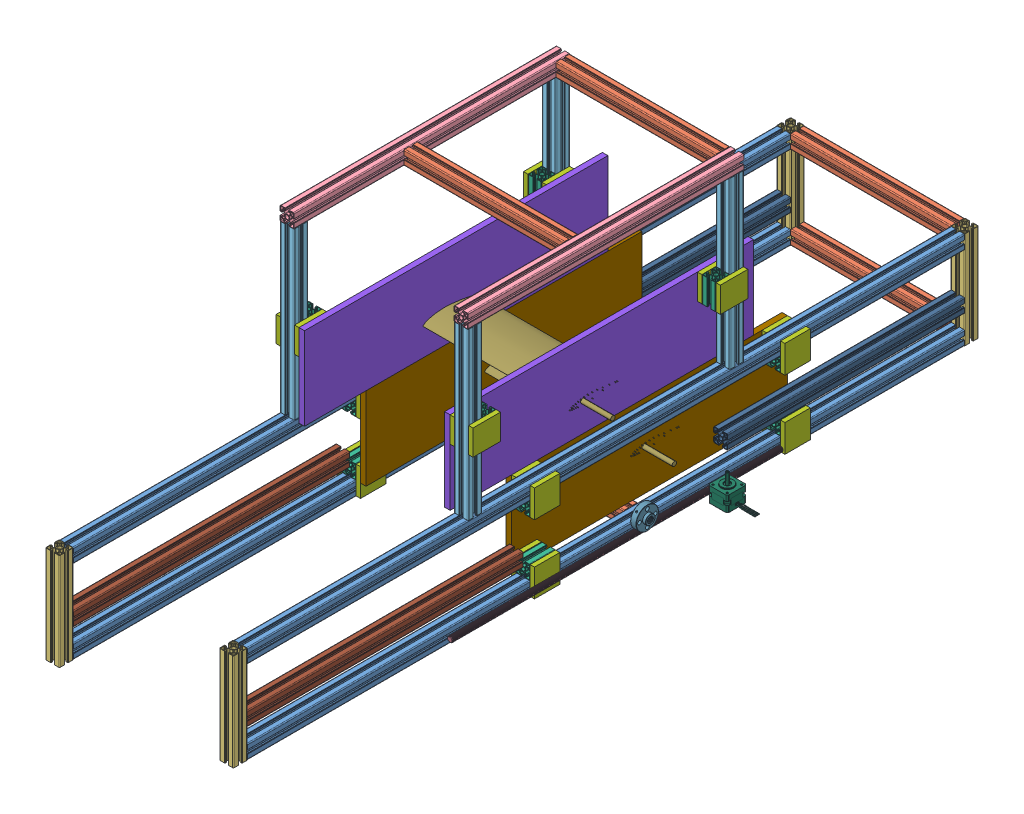
SolidWorks assembly Full Frame - Jack, configuration Default. Lengths in mm.
Overall size (567.71 501.2 1350.8).
82 component instances, 15 part files, 75 mates.
Components (placement in the parent):
- Stagger Frame-1: Stagger Frame [Default] at (96.6747 -83.0569 126.4787) size (340.8 175.8 1350.8)
  - Stagger - 1300x-1: Stagger - 1300x [Default] at (686.0911 649.1244 261.7798) size (25.4 25.4 1300)
  - Stagger - 1300x-2: Stagger - 1300x [Default] at (370.692 799.5238 261.7798) size (25.4 25.4 1300)
  - Stagger - 1300x-3: Stagger - 1300x [Default] at (686.0911 799.5238 261.7798) size (25.4 25.4 1300)
  - Stagger - 1300x-4: Stagger - 1300x [Default] at (370.692 649.1244 261.7798) size (25.4 25.4 1300)
  - Gap-220z-2: Gap-220z [Default] at (785.2806 799.5238 750.6531) x (0 0 1) z (-1 0 0) size (25.4 25.4 290)
  - Gap-220z-4: Gap-220z [Default] at (785.2806 649.1244 750.6531) x (0 0 1) z (-1 0 0) size (25.4 25.4 290)
  - Stagger 125y-5: Stagger 125y [Default] at (686.0911 880.052 750.6531) x (1 0 0) z (0 -1 0) size (25.4 25.4 175.8)
  - Stagger 125y-6: Stagger 125y [Default] at (370.692 880.052 750.6531) x (1 0 0) z (0 -1 0) size (25.4 25.4 175.8)
  - Stagger 125y-7: Stagger 125y [Default] at (370.692 568.5962 2076.0491) x (1 0 0) z (0 1 0) size (25.4 25.4 175.8)
  - Stagger 125y-8: Stagger 125y [Default] at (686.0911 568.5962 2076.0491) x (1 0 0) z (0 1 0) size (25.4 25.4 175.8)
- Gap Frame-1: Gap Frame [Default] at (534.4751 780.2503 996.128) size (340.8 325.4 500)
  - Gap-500x-1: Gap-500x [Default] at (248.2908 261.6156 100.7911) size (25.4 25.4 500)
  - Gap-500x-2: Gap-500x [Default] at (-67.1083 261.6156 100.7911) size (25.4 25.4 500)
  - Gap-300y-1: Gap-300y [Default] at (-67.1083 -166.8311 781.0023) x (1 0 0) z (0 1 0) size (25.4 25.4 300)
  - Gap-300y-2: Gap-300y [Default] at (-67.1083 -166.8311 306.4039) x (1 0 0) z (0 1 0) size (25.4 25.4 300)
  - Gap-300y-3: Gap-300y [Default] at (248.2908 364.6633 781.0023) x (1 0 0) z (0 -1 0) size (25.4 25.4 300)
  - Gap-300y-4: Gap-300y [Default] at (248.2908 364.6633 306.4039) x (1 0 0) z (0 -1 0) size (25.4 25.4 300)
  - Gap-220z-1: Gap-220z [Default] at (-166.2977 261.6156 581.8039) x (0 0 -1) z (1 0 0) size (25.4 25.4 290)
  - Gap-220z-2: Gap-220z [Default] at (347.4802 261.6156 306.4039) x (0 0 1) z (-1 0 0) size (25.4 25.4 290)
- Slider-1: Slider [Default] at (768.5368 912.233 1726.2246) x (1 0 0) z (0 -1 0) size (41.4 50 46)
  - Slider base-1: Slider base [Default] at (14.2291 25.5057 16.1181) size (25.4 25.4 46)
  - Slider Plate-1: Slider Plate [Default] at (34.9291 38.8389 53.7132) x (0 0 1) z (-1 0 0) size (46 50 8)
  - Slider Plate-2: Slider Plate [Default] at (1.5291 38.8389 53.7132) x (0 0 1) z (-1 0 0) size (46 50 8)
- Slider-2: Slider [Default] at (453.1377 912.233 1726.2246) x (1 0 0) z (0 -1 0) size (41.4 50 46)
  - Slider base-1: Slider base [Default] at (14.2291 25.5057 16.1181) size (25.4 25.4 46)
  - Slider Plate-1: Slider Plate [Default] at (34.9291 38.8389 53.7132) x (0 0 1) z (-1 0 0) size (46 50 8)
  - Slider Plate-2: Slider Plate [Default] at (1.5291 38.8389 53.7132) x (0 0 1) z (-1 0 0) size (46 50 8)
- Slider-3: Slider [Default] at (453.1377 798.5008 1353.4376) x (1 0 0) z (0 1 0) size (41.4 50 46)
  - Slider base-1: Slider base [Default] at (14.2291 25.5057 16.1181) size (25.4 25.4 46)
  - Slider Plate-1: Slider Plate [Default] at (34.9291 38.8389 53.7132) x (0 0 1) z (-1 0 0) size (46 50 8)
  - Slider Plate-2: Slider Plate [Default] at (1.5291 38.8389 53.7132) x (0 0 1) z (-1 0 0) size (46 50 8)
- Slider-4: Slider [Default] at (768.5368 798.5008 1353.4376) x (1 0 0) z (0 1 0) size (41.4 50 46)
  - Slider base-1: Slider base [Default] at (14.2291 25.5057 16.1181) size (25.4 25.4 46)
  - Slider Plate-1: Slider Plate [Default] at (34.9291 38.8389 53.7132) x (0 0 1) z (-1 0 0) size (46 50 8)
  - Slider Plate-2: Slider Plate [Default] at (1.5291 38.8389 53.7132) x (0 0 1) z (-1 0 0) size (46 50 8)
- Gap Endplate-1: Gap Endplate [Default] at (498.0668 949.276 1602.5657) x (0 0 1) z (-1 0 0) size (550 150 10)
- Gap Endplate-2: Gap Endplate [Default] at (752.0659 949.276 1425.495) x (0 0 -1) z (1 0 0) size (550 150 10)
- Slider-5: Slider [Default] at (768.5368 665.5612 1597.602) size (41.4 50 46)
  - Slider base-1: Slider base [Default] at (14.2291 25.5057 16.1181) size (25.4 25.4 46)
  - Slider Plate-1: Slider Plate [Default] at (34.9291 38.8389 53.7132) x (0 0 1) z (-1 0 0) size (46 50 8)
  - Slider Plate-2: Slider Plate [Default] at (1.5291 38.8389 53.7132) x (0 0 1) z (-1 0 0) size (46 50 8)
- Slider-6: Slider [Default] at (453.1377 665.5612 1597.602) size (41.4 50 46)
  - Slider base-1: Slider base [Default] at (14.2291 25.5057 16.1181) size (25.4 25.4 46)
  - Slider Plate-1: Slider Plate [Default] at (34.9291 38.8389 53.7132) x (0 0 1) z (-1 0 0) size (46 50 8)
  - Slider Plate-2: Slider Plate [Default] at (1.5291 38.8389 53.7132) x (0 0 1) z (-1 0 0) size (46 50 8)
- Slider-7: Slider [Default] at (453.1377 616.9732 1711.3342) x (1 0 0) z (0 0 -1) size (41.4 50 46)
  - Slider base-1: Slider base [Default] at (14.2291 25.5057 16.1181) size (25.4 25.4 46)
  - Slider Plate-1: Slider Plate [Default] at (34.9291 38.8389 53.7132) x (0 0 1) z (-1 0 0) size (46 50 8)
  - Slider Plate-2: Slider Plate [Default] at (1.5291 38.8389 53.7132) x (0 0 1) z (-1 0 0) size (46 50 8)
- Slider-8: Slider [Default] at (768.5368 616.9732 1711.3342) x (1 0 0) z (0 0 -1) size (41.4 50 46)
  - Slider base-1: Slider base [Default] at (14.2291 25.5057 16.1181) size (25.4 25.4 46)
  - Slider Plate-1: Slider Plate [Default] at (34.9291 38.8389 53.7132) x (0 0 1) z (-1 0 0) size (46 50 8)
  - Slider Plate-2: Slider Plate [Default] at (1.5291 38.8389 53.7132) x (0 0 1) z (-1 0 0) size (46 50 8)
- Stagger Endplate-1: Stagger Endplate [Default] at (498.0668 653.3669 1427.4681) x (0 0 1) z (-1 0 0) size (500 150 10)
- Slider-9: Slider [Default] at (453.1377 665.5612 1143.602) size (41.4 50 46)
  - Slider base-1: Slider base [Default] at (14.2291 25.5057 16.1181) size (25.4 25.4 46)
  - Slider Plate-1: Slider Plate [Default] at (34.9291 38.8389 53.7132) x (0 0 1) z (-1 0 0) size (46 50 8)
  - Slider Plate-2: Slider Plate [Default] at (1.5291 38.8389 53.7132) x (0 0 1) z (-1 0 0) size (46 50 8)
- Slider-10: Slider [Default] at (453.1377 616.9732 1257.3342) x (1 0 0) z (0 0 -1) size (41.4 50 46)
  - Slider base-1: Slider base [Default] at (14.2291 25.5057 16.1181) size (25.4 25.4 46)
  - Slider Plate-1: Slider Plate [Default] at (34.9291 38.8389 53.7132) x (0 0 1) z (-1 0 0) size (46 50 8)
  - Slider Plate-2: Slider Plate [Default] at (1.5291 38.8389 53.7132) x (0 0 1) z (-1 0 0) size (46 50 8)
- Slider-11: Slider [Default] at (768.5368 616.9732 1257.3342) x (1 0 0) z (0 0 -1) size (41.4 50 46)
  - Slider base-1: Slider base [Default] at (14.2291 25.5057 16.1181) size (25.4 25.4 46)
  - Slider Plate-1: Slider Plate [Default] at (34.9291 38.8389 53.7132) x (0 0 1) z (-1 0 0) size (46 50 8)
  - Slider Plate-2: Slider Plate [Default] at (1.5291 38.8389 53.7132) x (0 0 1) z (-1 0 0) size (46 50 8)
- Slider-12: Slider [Default] at (768.5368 665.5612 1143.602) size (41.4 50 46)
  - Slider base-1: Slider base [Default] at (14.2291 25.5057 16.1181) size (25.4 25.4 46)
  - Slider Plate-1: Slider Plate [Default] at (34.9291 38.8389 53.7132) x (0 0 1) z (-1 0 0) size (46 50 8)
  - Slider Plate-2: Slider Plate [Default] at (1.5291 38.8389 53.7132) x (0 0 1) z (-1 0 0) size (46 50 8)
- Stagger Endplate-2: Stagger Endplate [Default] at (762.0659 653.3669 1427.4681) x (0 0 1) z (-1 0 0) size (500 150 10)
- stagger holder short-1: stagger holder short [Default] at (782.7659 616.8674 889.8319) size (25.4 25.4 429.35)
- stagger holder short-2: stagger holder short [Default] at (467.3668 616.8674 889.8319) size (25.4 25.4 429.35)
- stagger holder long-1: stagger holder long [Default] at (467.3668 616.8674 1689.0278) size (25.4 25.4 500.8)
- stagger holder long-2: stagger holder long [Default] at (781.6523 616.8674 1689.0278) size (25.4 25.4 500.8)
- Airfoil-1: Airfoil [Default] at (624.5659 650.3067 1462.4681) x (0 0 -1) z (1 0 0) size (100.18 14.48 385)
- Airfoil-2: Airfoil [Default] at (624.5659 777.8269 1574.0303) x (0 0 -1) z (1 0 0) size (100.18 14.48 385)
- Gap-220z-1: Gap-220z [Default] at (881.9553 566.0674 1469.6132) x (0 0 1) z (-1 0 0) size (25.4 25.4 290)
- 7549K72_Lead Screw-1: 7549K72_Lead Screw [7549K72] at (812.6839 576.4626 1540.2399) size (10.51 10.35 601.83)
- 7549K16_Precision Acme Flange Nut-1: 7549K16_Precision Acme Flange Nut [7549K16] at (878.0687 663.8356 1557.7374) size (16.19 40.64 40.64)
- SY35ST28-0504A (1).step-1: SY35ST28-0504A (1).step [Default] at (945.5426 701.0441 1469.9684) size (71.83 49 35.2)
Mates (geometry in assembly coordinates):
- Coincident1: coincident anti-aligned: plane of Stagger Frame-1/Stagger - 1300x-2 through (456.3601 729.1669 2189.8278) normal (0 1 0); plane of Gap Frame-1/Gap-300y-2 through (467.3668 729.1669 1302.5319) normal (0 -1 0)
- Coincident3: coincident: line of Stagger Frame-1/Stagger - 1300x-2 through (478.3735 729.1669 2189.8278) axis (0 0 -1); point of Gap Frame-1/Gap-300y-2
- Coincident6: coincident: line of Stagger Frame-1/Stagger - 1300x-2 through (456.3601 729.1669 2189.8278) axis (0 0 -1); point of Gap Frame-1/Gap-300y-1
- Distance1: distance = 400 mm: line of Gap Frame-1/Gap-300y-2 through (463.8108 729.1669 1289.8319) axis (-1 0 0); line of Stagger Frame-1/Stagger - 1300x-2 through (463.8108 729.1669 889.8319) axis (-1 0 0)
- Coincident7: coincident anti-aligned: plane of Gap Frame-1/Gap-300y-3 through (770.0659 729.1669 1766.1237) normal (-1 0 0); plane of Slider-1/Slider Plate-2 through (770.0659 858.5198 1765.0635) normal (1 0 0)
- Parallel2: parallel aligned: line of Gap Frame-1/Gap-500x-1 through (770.9126 1031.4237 1789.8303) axis (0 0 -1); line of Slider-1/Slider Plate-2 through (762.0659 878.3669 1789.0303) axis (0 0 -1)
- Coincident8: coincident anti-aligned: plane of Gap Frame-1/Gap-300y-3 through (793.7725 729.1669 1764.4303) normal (0 0 -1); plane of Slider-1/Slider base-1 through (793.7725 832.367 1764.4303) normal (0 0 1)
- Coincident9: coincident anti-aligned: plane of Gap Frame-1/Gap-300y-1 through (480.0668 1029.166 1766.1237) normal (1 0 0); plane of Slider-2/Slider Plate-1 through (480.0668 858.5198 1765.0635) normal (-1 0 0)
- Parallel3: parallel aligned: line of Gap Frame-1/Gap-500x-2 through (479.2201 1031.4237 1789.8303) axis (0 0 -1); line of Slider-2/Slider Plate-1 through (488.0668 878.3669 1789.0303) axis (0 0 -1)
- Coincident10: coincident anti-aligned: plane of Gap Frame-1/Gap-300y-1 through (478.3735 1029.166 1764.4303) normal (0 0 -1); plane of Slider-2/Slider base-1 through (478.3735 832.367 1764.4303) normal (0 0 1)
- Distance3: distance = 0 mm: line of Slider-2/Slider Plate-1 through (480.0668 878.3669 1739.0303) axis (1 0 0); line of Slider-1/Slider Plate-2 through (762.0659 878.3669 1739.0303) axis (1 0 0)
- Coincident11: coincident anti-aligned: plane of Gap Frame-1/Gap-300y-2 through (480.0668 1029.166 1313.5385) normal (1 0 0); plane of Slider-3/Slider Plate-1 through (480.0668 852.214 1314.5987) normal (-1 0 0)
- Parallel4: parallel aligned: line of Gap Frame-1/Gap-500x-1 through (795.4659 1030.8593 1789.8303) axis (0 0 -1); line of Slider-3/Slider Plate-1 through (488.0668 878.3669 1340.6319) axis (0 0 -1)
- Coincident12: coincident anti-aligned: plane of Gap Frame-1/Gap-300y-2 through (478.3735 1029.166 1315.2319) normal (0 0 1); plane of Slider-3/Slider base-1 through (478.3735 878.3668 1315.2319) normal (0 0 -1)
- Distance4: distance = 0 mm: line of Slider-3/Slider Plate-1 through (488.0668 878.3669 1340.6319) axis (0 0 -1); line of Slider-2/Slider Plate-1 through (488.0668 878.3669 1789.0303) axis (0 0 -1)
- Coincident13: coincident anti-aligned: plane of Gap Frame-1/Gap-300y-4 through (770.0659 729.1669 1313.5385) normal (-1 0 0); plane of Slider-4/Slider Plate-2 through (770.0659 852.214 1314.5987) normal (1 0 0)
- Parallel5: parallel aligned: line of Gap Frame-1/Gap-500x-1 through (770.0659 1030.8593 1789.8303) axis (0 0 -1); line of Slider-4/Slider Plate-2 through (762.0659 878.3669 1340.6319) axis (0 0 -1)
- Coincident14: coincident anti-aligned: plane of Gap Frame-1/Gap-300y-4 through (771.7592 729.1669 1315.2319) normal (0 0 1); plane of Slider-4/Slider base-1 through (771.7592 878.3668 1315.2319) normal (0 0 -1)
- Distance5: distance = 0 mm: line of Slider-3/Slider Plate-1 through (480.0668 878.3669 1340.6319) axis (1 0 0); line of Slider-4/Slider Plate-2 through (762.0659 878.3669 1340.6319) axis (1 0 0)
- Coincident15: coincident anti-aligned: plane of Slider-2/Slider Plate-1 through (488.0668 858.5198 1765.0635) normal (1 0 0); plane of Gap Endplate-1 through (488.0668 949.276 1602.5657) normal (-1 0 0)
- Coincident16: coincident aligned: line of Slider-2/Slider Plate-1 through (488.0668 832.3669 1789.0303) axis (0 1 0); line of Gap Endplate-1 through (488.0668 728.3669 1789.0303) axis (0 1 0)
- Coincident17: coincident aligned: line of Slider-2/Slider Plate-1 through (488.0668 878.3669 1789.0303) axis (0 0 -1); line of Gap Endplate-1 through (488.0668 878.3669 1789.0303) axis (0 0 -1)
- Coincident18: coincident anti-aligned: plane of Slider-1/Slider Plate-2 through (762.0659 858.5198 1765.0635) normal (-1 0 0); plane of Gap Endplate-2 through (762.0659 949.276 1425.495) normal (1 0 0)
- Coincident19: coincident anti-aligned: line of Slider-1/Slider Plate-2 through (762.0659 832.3669 1789.0303) axis (0 1 0); line of Gap Endplate-2 through (762.0659 878.3669 1789.0303) axis (0 -1 0)
- Coincident20: coincident anti-aligned: line of Slider-1/Slider Plate-2 through (762.0659 878.3669 1789.0303) axis (0 0 -1); line of Gap Endplate-2 through (762.0659 878.3669 1239.0303) axis (0 0 1)
- Coincident21: coincident anti-aligned: plane of Stagger Frame-1/Stagger - 1300x-3 through (770.0659 705.4602 2189.8278) normal (-1 0 0); plane of Slider-5/Slider Plate-2 through (770.0659 704.4001 1651.3151) normal (1 0 0)
- Coincident22: coincident anti-aligned: plane of Stagger Frame-1/Stagger - 1300x-3 through (793.7725 703.7669 2189.8278) normal (0 -1 0); plane of Slider-5/Slider base-1 through (793.7725 703.7669 1677.4679) normal (0 1 0)
- Coincident23: coincident anti-aligned: plane of Stagger Frame-1/Stagger - 1300x-2 through (454.6668 705.4602 2189.8278) normal (-1 0 0); plane of Slider-6/Slider Plate-2 through (454.6668 704.4001 1651.3151) normal (1 0 0)
- Coincident24: coincident anti-aligned: plane of Stagger Frame-1/Stagger - 1300x-2 through (478.3735 703.7669 2189.8278) normal (0 -1 0); plane of Slider-6/Slider base-1 through (478.3735 703.7669 1677.4679) normal (0 1 0)
- Distance6: distance = 0 mm: line of Slider-6/Slider Plate-1 through (480.0668 728.3669 1677.4681) axis (1 0 0); line of Slider-5/Slider Plate-2 through (762.0659 728.3669 1677.4681) axis (1 0 0)
- Coincident25: coincident anti-aligned: plane of Stagger Frame-1/Stagger - 1300x-4 through (454.6668 577.0741 2189.8278) normal (-1 0 0); plane of Slider-7/Slider Plate-2 through (454.6668 578.1343 1657.621) normal (1 0 0)
- Coincident26: coincident anti-aligned: plane of Stagger Frame-1/Stagger - 1300x-4 through (478.3735 578.7674 2189.8278) normal (0 1 0); plane of Slider-7/Slider base-1 through (478.3735 578.7674 1631.4682) normal (0 -1 0)
- Distance11: distance = 0 mm: line of Slider-7/Slider Plate-2 through (446.6668 554.1674 1677.4681) axis (0 1 0); line of Slider-6/Slider Plate-2 through (446.6668 678.3669 1677.4681) axis (0 1 0)
- Coincident27: coincident anti-aligned: plane of Stagger Frame-1/Stagger - 1300x-1 through (770.0659 577.0741 2189.8278) normal (-1 0 0); plane of Slider-8/Slider Plate-2 through (770.0659 578.1343 1657.621) normal (1 0 0)
- Coincident28: coincident anti-aligned: plane of Stagger Frame-1/Stagger - 1300x-1 through (793.7725 578.7674 2189.8278) normal (0 1 0); plane of Slider-8/Slider base-1 through (793.7725 578.7674 1631.4682) normal (0 -1 0)
- Coincident29: coincident aligned: line of Slider-5/Slider Plate-2 through (762.0659 678.3669 1677.4681) axis (0 1 0); line of Slider-8/Slider Plate-2 through (762.0659 554.1674 1677.4681) axis (0 1 0)
- Coincident30: coincident anti-aligned: plane of Slider-6/Slider Plate-1 through (488.0668 704.4001 1651.3151) normal (1 0 0); plane of Stagger Endplate-1 through (488.0668 653.3669 1427.4681) normal (-1 0 0)
- Coincident33: coincident aligned: line of Slider-6/Slider Plate-1 through (488.0668 678.3669 1677.4681) axis (0 1 0); line of Stagger Endplate-1 through (488.0668 578.3669 1677.4681) axis (0 1 0)
- Coincident35: coincident aligned: line of Slider-6/Slider Plate-1 through (488.0668 728.3669 1677.4681) axis (0 0 -1); line of Stagger Endplate-1 through (488.0668 728.3669 1677.4681) axis (0 0 -1)
- Coincident36: coincident anti-aligned: plane of Stagger Frame-1/Stagger - 1300x-2 through (454.6668 705.4602 2189.8278) normal (-1 0 0); plane of Slider-9/Slider Plate-2 through (454.6668 704.4001 1197.3151) normal (1 0 0)
- Coincident37: coincident anti-aligned: plane of Stagger Frame-1/Stagger - 1300x-2 through (456.3601 703.7669 2189.8278) normal (0 -1 0); plane of Slider-9/Slider base-1 through (456.3601 703.7669 1223.4679) normal (0 1 0)
- Coincident38: coincident aligned: line of Stagger Endplate-1 through (488.0668 728.3669 1677.4681) axis (0 0 -1); line of Slider-9/Slider Plate-1 through (488.0668 728.3669 1223.4681) axis (0 0 -1)
- Coincident39: coincident aligned: line of Stagger Endplate-1 through (488.0668 728.3669 1177.4681) axis (0 -1 0); line of Slider-9/Slider Plate-1 through (488.0668 728.3669 1177.4681) axis (0 -1 0)
- Coincident40: coincident anti-aligned: plane of Stagger Frame-1/Stagger - 1300x-4 through (480.0668 555.0608 2189.8278) normal (1 0 0); plane of Slider-10/Slider Plate-1 through (480.0668 578.1343 1203.621) normal (-1 0 0)
- Coincident41: coincident anti-aligned: plane of Stagger Frame-1/Stagger - 1300x-4 through (456.3601 578.7674 2189.8278) normal (0 1 0); plane of Slider-10/Slider base-1 through (456.3601 578.7674 1177.4682) normal (0 -1 0)
- Coincident42: coincident aligned: line of Stagger Endplate-1 through (488.0668 728.3669 1177.4681) axis (0 -1 0); line of Slider-10/Slider Plate-1 through (488.0668 604.1674 1177.4681) axis (0 -1 0)
- Coincident43: coincident anti-aligned: plane of Stagger Frame-1/Stagger - 1300x-3 through (770.0659 727.4736 2189.8278) normal (-1 0 0); plane of Slider-12/Slider Plate-2 through (770.0659 704.4001 1197.3151) normal (1 0 0)
- Coincident44: coincident anti-aligned: plane of Stagger Frame-1/Stagger - 1300x-3 through (771.7592 703.7669 2189.8278) normal (0 -1 0); plane of Slider-12/Slider base-1 through (771.7592 703.7669 1223.4679) normal (0 1 0)
- Coincident45: coincident anti-aligned: plane of Stagger Frame-1/Stagger - 1300x-1 through (770.0659 577.0741 2189.8278) normal (-1 0 0); plane of Slider-11/Slider Plate-2 through (770.0659 578.1343 1203.621) normal (1 0 0)
- Coincident46: coincident anti-aligned: plane of Stagger Frame-1/Stagger - 1300x-1 through (771.7592 578.7674 2189.8278) normal (0 1 0); plane of Slider-11/Slider base-1 through (771.7592 578.7674 1177.4682) normal (0 -1 0)
- Distance20: distance = 0 mm: line of Slider-11/Slider Plate-1 through (803.4659 604.1674 1177.4681) axis (0 -1 0); line of Slider-12/Slider Plate-1 through (803.4659 728.3669 1177.4681) axis (0 -1 0)
- Distance21: distance = 0 mm: line of Slider-11/Slider Plate-2 through (762.0659 604.1674 1177.4681) axis (1 0 0); line of Slider-10/Slider Plate-1 through (480.0668 604.1674 1177.4681) axis (1 0 0)
- Coincident48: coincident anti-aligned: plane of Slider-5/Slider Plate-2 through (762.0659 704.4001 1651.3151) normal (-1 0 0); plane of Stagger Endplate-2 through (762.0659 653.3669 1427.4681) normal (1 0 0)
- Coincident50: coincident aligned: line of Slider-5/Slider Plate-2 through (762.0659 728.3669 1677.4681) axis (0 0 -1); line of Stagger Endplate-2 through (762.0659 728.3669 1677.4681) axis (0 0 -1)
- Coincident83: coincident anti-aligned: plane of Stagger Frame-1/Stagger 125y-6 through (456.3601 553.3674 889.8319) normal (0 0 1); plane of stagger holder short-2 through (467.3668 616.8674 889.8319) normal (0 0 -1)
- Coincident84: coincident anti-aligned: plane of Slider-10/Slider base-1 through (456.3601 604.1674 1177.4682) normal (0 1 0); plane of stagger holder short-2 through (456.3601 604.1674 1319.1819) normal (0 -1 0)
- Coincident85: coincident: point of Slider-10/Slider base-1; line of stagger holder short-2 through (478.3735 604.1674 1319.1819) axis (0 0 -1)
- Coincident89: coincident anti-aligned: plane of Stagger Frame-1/Stagger 125y-5 through (793.7725 553.3674 889.8319) normal (0 0 1); plane of stagger holder short-1 through (782.7659 616.8674 889.8319) normal (0 0 -1)
- Coincident90: coincident anti-aligned: plane of Slider-11/Slider base-1 through (771.7592 604.1674 1177.4682) normal (0 1 0); plane of stagger holder short-1 through (771.7592 604.1674 1319.1819) normal (0 -1 0)
- Coincident91: coincident: point of Slider-11/Slider base-1; line of stagger holder short-1 through (771.7592 604.1674 1319.1819) axis (0 0 -1)
- Coincident97: coincident anti-aligned: plane of Stagger Frame-1/Stagger 125y-7 through (478.3735 729.1669 2189.8278) normal (0 0 -1); plane of stagger holder long-1 through (467.3668 616.8674 2189.8278) normal (0 0 1)
- Coincident98: coincident anti-aligned: plane of Slider-7/Slider base-1 through (456.3601 604.1674 1631.4682) normal (0 1 0); plane of stagger holder long-1 through (456.3601 604.1674 2189.8278) normal (0 -1 0)
- Coincident99: coincident: point of Slider-7/Slider base-1; line of stagger holder long-1 through (456.3601 604.1674 2189.8278) axis (0 0 -1)
- Coincident100: coincident anti-aligned: plane of Stagger Frame-1/Stagger 125y-8 through (793.7725 729.1669 2189.8278) normal (0 0 -1); plane of stagger holder long-2 through (781.6523 616.8674 2189.8278) normal (0 0 1)
- Coincident101: coincident anti-aligned: plane of Slider-8/Slider base-1 through (793.7725 604.1674 1631.4682) normal (0 1 0); plane of stagger holder long-2 through (792.659 604.1674 2189.8278) normal (0 -1 0)
- Coincident110: coincident anti-aligned: plane of Gap Endplate-2 through (762.0659 728.3669 1789.0303) normal (0 -1 0); plane of Stagger Endplate-2 through (752.0659 728.3669 1177.4681) normal (0 1 0)
- Coincident114: coincident anti-aligned: plane of Gap Endplate-2 through (752.0659 949.276 1425.495) normal (-1 0 0); plane of Airfoil-2 through (752.0659 778.9515 1573.5335) normal (1 0 0)
- Distance48: distance = 52.16 mm: plane of assembly through (624.5659 780.5269 1574.0303) normal (0 1 0); plane of assembly; plane of Stagger Endplate-2 through (752.0659 728.3669 1177.4681) normal (0 1 0)
- Distance49: distance = 240 mm: plane of assembly through (624.5659 777.8269 1549.0303) normal (0 0 -1); plane of assembly; plane of Gap Endplate-2 through (762.0659 728.3669 1789.0303) normal (0 0 1)
- Coincident115: coincident anti-aligned: plane of Stagger Endplate-2 through (752.0659 653.3669 1427.4681) normal (-1 0 0); plane of Airfoil-1 through (752.0659 651.4313 1461.9713) normal (1 0 0)
- Distance50: distance = 240 mm: plane of assembly through (624.5659 650.3067 1437.4681) normal (0 0 -1); plane of assembly; plane of Stagger Endplate-2 through (752.0659 578.3669 1677.4681) normal (0 0 1)
- Coincident116: coincident aligned: plane of Stagger Endplate-1 through (488.0668 578.3669 1677.4681) normal (0 0 1); plane of Stagger Endplate-2 through (752.0659 578.3669 1677.4681) normal (0 0 1)
- Coincident117: coincident anti-aligned: plane of Stagger Frame-1/Stagger - 1300x-4 through (480.0668 577.0741 2189.8278) normal (1 0 0); plane of Gap-220z-1 through (480.0668 566.0674 1469.6132) normal (-1 0 0)
- Coincident118: coincident aligned: plane of Stagger Frame-1/Stagger - 1300x-1 through (771.7592 553.3674 2189.8278) normal (0 -1 0); plane of Gap-220z-1 through (480.0668 553.3674 1480.6198) normal (0 -1 0)
- Distance51: distance = 567.0813 mm anti-aligned: plane of Gap-220z-1 through (480.0668 577.0741 1456.9132) normal (0 0 -1); plane of Stagger Frame-1/Gap-220z-4 through (480.0668 555.0608 889.8319) normal (0 0 1)
